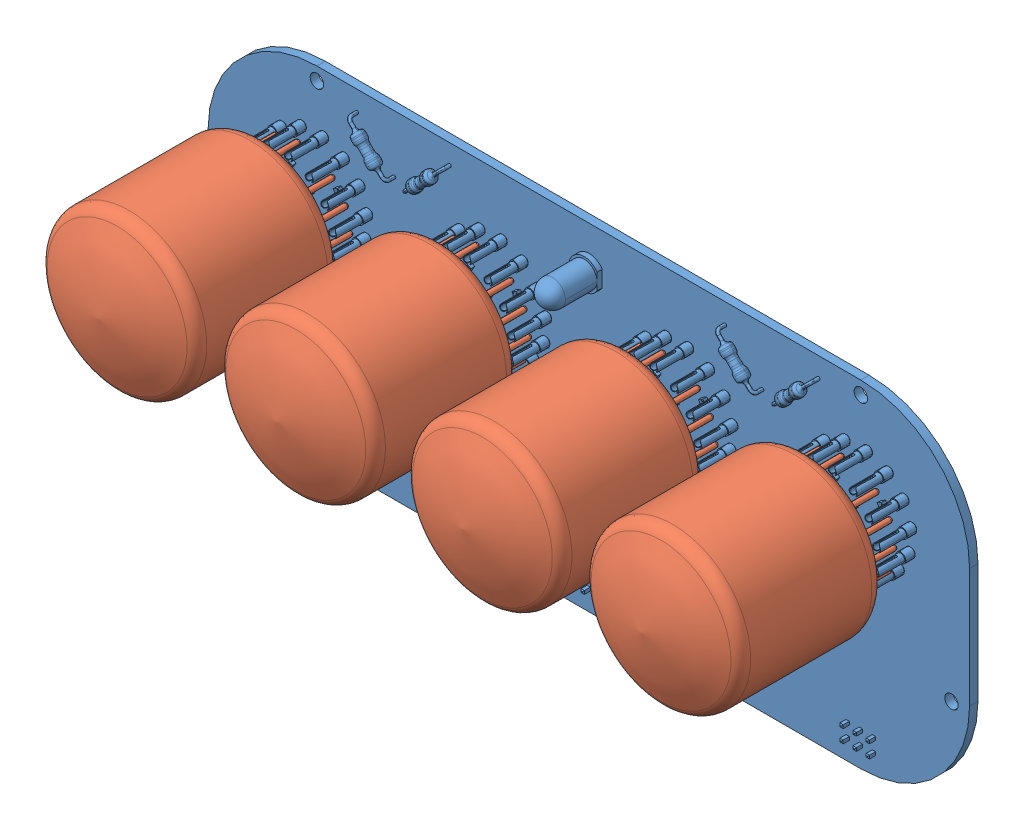
SolidWorks assembly nixi_ clock_asm, configuration Default. Lengths in mm.
Overall size (147 65 52.55).
9 component instances, 6 part files, 18 mates.
Components (placement in the parent):
- nixi_tube.step-1: nixi_tube.step [Default] at (0 0 11) x (-1 0 0) z (0 0 -1) size (147 65 19.82)
- nixie_clock_holder.step-1: nixie_clock_holder.step [Default] at (0 0 41) x (-1 0 0) z (0 0 -1) size (147 70 1.62) (hidden)
- nixi_ clock_cpu.step-2: nixi_ clock_cpu.step [Default] at origin size (151.78 65 13.45) (hidden)
- in-4_nixie_tube-5: in-4_nixie_tube [Default] at (-52.5 0 39) size (30 30 42)
- in-4_nixie_tube-6: in-4_nixie_tube [Default] at (-18 0 39) size (30 30 42)
- in-4_nixie_tube-7: in-4_nixie_tube [Default] at (18 0 39) size (30 30 42)
- in-4_nixie_tube-8: in-4_nixie_tube [Default] at (52.5 0 39) size (30 30 42)
- box_rear-1: box_rear [Default] at (0 -12 -8.5) size (155 76 26.25) (hidden)
- box_top-1: box_top [Default] at (0 -12 43.5) x (-1 0 0) z (0 0 -1) size (155.1 76.05 34.49) (hidden)
Mates (geometry in assembly coordinates):
- Coincidente14: coincident aligned: plane of nixi_ clock_cpu.step-2 through (0 0 0) normal (0 0 1)
- Distanza5: distance = 11 mm anti-aligned: plane of nixi_tube.step-1 through (0 0 11) normal (0 0 -1)
- Coincidente15: coincident aligned: plane of nixi_tube.step-1 through (0 0 11) normal (0 1 0)
- Coincidente16: coincident anti-aligned: plane of nixi_tube.step-1 through (0 0 11) normal (-1 0 0)
- Coincidente17: coincident aligned: plane of nixi_ clock_cpu.step-2 through (0 0 0) normal (0 1 0)
- Coincidente18: coincident anti-aligned: plane of nixi_tube.step-1 through (0 0 11) normal (-1 0 0); plane of nixi_ clock_cpu.step-2 through (0 0 0) normal (1 0 0)
- Coincidente19: coincident aligned: plane of nixie_clock_holder.step-1 through (0 0 41) normal (0 1 0)
- Coincidente20: coincident anti-aligned: plane of nixie_clock_holder.step-1 through (0 0 41) normal (-1 0 0)
- Distanza6: distance = 30 mm aligned: plane of nixi_tube.step-1 through (0 0 11) normal (0 0 -1); plane of nixie_clock_holder.step-1 through (0 0 41) normal (0 0 -1)
- Coincidente22: coincident aligned: plane of nixi_tube.step-1 through (0 0 11) normal (0 1 0); plane of in-4_nixie_tube-5 through (-52.5 0 39) normal (0 1 0)
- Distanza7: distance = 52.5 mm aligned: plane of in-4_nixie_tube-5 through (-52.5 0 39) normal (1 0 0)
- Distanza8: distance = 28 mm anti-aligned: plane of in-4_nixie_tube-5 through (-52.5 0 39) normal (0 0 1); plane of nixi_tube.step-1 through (0 0 11) normal (0 0 -1)
- Distanza9: distance = 12 mm: plane of assembly through (0 0 0) normal (0 1 0); plane of assembly; plane of box_rear-1 through (0 -12 -8.5) normal (0 1 0)
- Coincidente26: coincident aligned: plane of box_rear-1 through (0 -12 -8.5) normal (1 0 0)
- Distanza10: distance = 8.5 mm aligned: plane of box_rear-1 through (0 -12 -8.5) normal (0 0 1)
- Distanza11: distance = 12 mm: plane of assembly through (0 0 0) normal (0 1 0); plane of assembly; plane of box_top-1 through (0 -12 43.5) normal (0 1 0)
- Coincidente27: coincident anti-aligned: plane of box_top-1 through (0 -12 43.5) normal (-1 0 0)
- Coincidente28: coincident anti-aligned: plane of box_rear-1 through (52.4992 -0.5008 17.5) normal (0 0 1); plane of box_top-1 through (-52.4992 -0.5008 17.5) normal (0 0 -1)
